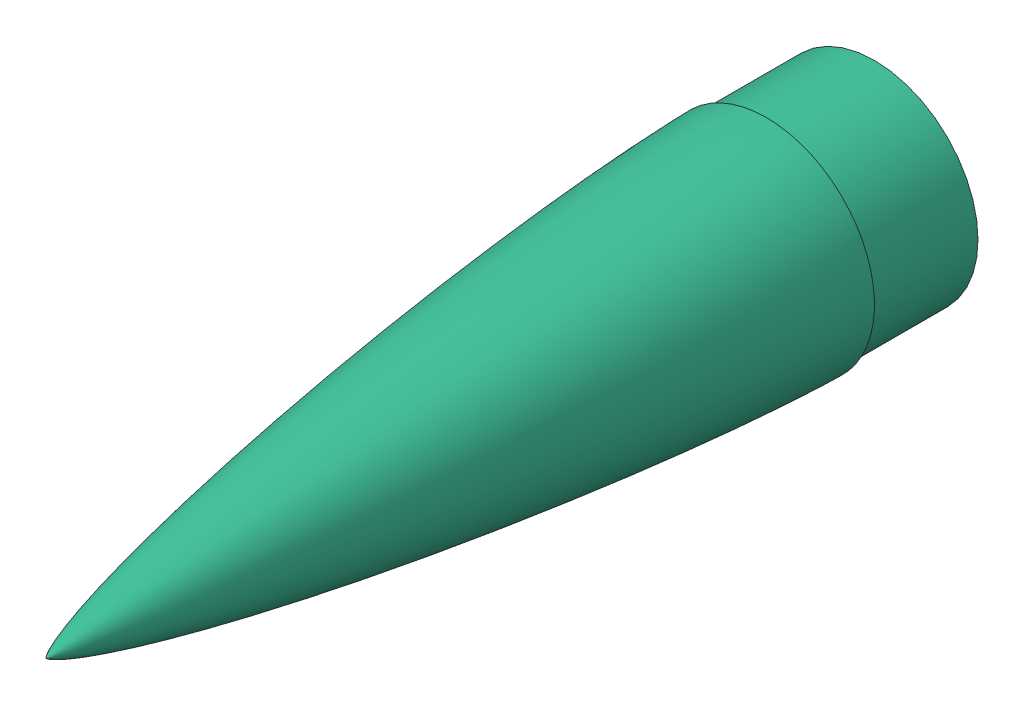
SolidWorks assembly Nosecone Assembly, configuration Default. Lengths in mm.
Overall size (152.4 152.4 590.12).
7 component instances, 7 part files, 13 mates.
Components (placement in the parent):
- 3112T31_Zinc-Plated Steel Round Eye Nut - for Lifting-1: 3112T31_Zinc-Plated Steel Round Eye Nut - for Lifting [3112T31] at (-62.4913 0 510.0607) x (0.999986 0.005369 0) z (-0.005369 0.999986 0) size (36.07 36.46 19.73)
- 90107A029_316 Stainless Steel Washer-1: 90107A029_316 Stainless Steel Washer [90107A029] at (-62.4913 0 546.986) size (15.88 15.88 1.27)
- 90322A658_High-Strength Steel Threaded Rod-1: 90322A658_High-Strength Steel Threaded Rod [90322A658] at (-62.4913 0 790.1916) x (-0.708492 -0.705719 0) z (0 0 1) size (7.33 6.42 560.63)
- 90630A110_High-Strength Steel Nylon-Insert Locknut-1: 90630A110_High-Strength Steel Nylon-Insert Locknut [90630A110] at (-62.4913 0 547.621) x (1 0 0) z (0 -1 0) size (11.11 8.31 12.83)
- 95462A029_Medium-Strength Steel Hex Nut-1: 95462A029_Medium-Strength Steel Hex Nut [95462A029] at (-62.4913 0 530.8728) x (0.99999 0.004487 0) z (0 0 1) size (11.11 12.75 6.32)
- LD-20-1: LD-20 [Default] at (-62.4913 0 1082.1485) x (0 0 -1) z (1 0 0) size (584.2 152.4 152.4)
- Nosecone Avionics Bulkhead-1: Nosecone Avionics Bulkhead [Default] at (-62.4913 0 546.351) x (1 0 0) z (0 1 0) size (139.7 12.7 139.7)
Mates (geometry in assembly coordinates):
- Concentric1: concentric anti-aligned: circle of 90322A658_High-Strength Steel Threaded Rod-1; circle of LD-20-1
- Coincident2: coincident aligned: plane of LD-20-1 through (-62.4913 0 1082.1485) normal (0 1 0)
- Tangent3: tangent: circle of 90322A658_High-Strength Steel Threaded Rod-1; face of LD-20-1
- Concentric2: concentric anti-aligned: cylinder of 90630A110_High-Strength Steel Nylon-Insert Locknut-1; cylinder of LD-20-1 through (-62.4913 0 574.1485) axis (0 0 -1) radius 69.85
- Coincident4: coincident anti-aligned: plane of 90107A029_316 Stainless Steel Washer-1 through (-62.4913 0 547.621) normal (0 0 1); plane of 90630A110_High-Strength Steel Nylon-Insert Locknut-1 through (-56.9351 3.2079 547.621) normal (0 0 -1)
- Concentric3: concentric aligned: circle of 90107A029_316 Stainless Steel Washer-1; circle of 90630A110_High-Strength Steel Nylon-Insert Locknut-1
- Concentric4: concentric aligned: circle of 3112T31_Zinc-Plated Steel Round Eye Nut - for Lifting-1; circle of 95462A029_Medium-Strength Steel Hex Nut-1
- Concentric5: concentric anti-aligned: cylinder of LD-20-1 through (-62.4913 0 574.1485) axis (0 0 -1) radius 69.85; cylinder of Nosecone Avionics Bulkhead-1 through (-62.4913 0 533.651) axis (0 0 1) radius 69.85
- Coincident6: coincident anti-aligned: plane of 90107A029_316 Stainless Steel Washer-1 through (-62.4913 0 546.351) normal (0 0 -1); plane of Nosecone Avionics Bulkhead-1 through (-62.4913 0 546.351) normal (0 0 1)
- Coincident7: coincident anti-aligned: plane of 95462A029_Medium-Strength Steel Hex Nut-1 through (-62.4913 0 533.651) normal (0 0 1); plane of Nosecone Avionics Bulkhead-1 through (-62.4913 0 533.651) normal (0 0 -1)
- Concentric6: concentric aligned: circle of 95462A029_Medium-Strength Steel Hex Nut-1; circle of Nosecone Avionics Bulkhead-1
- Coincident11: coincident anti-aligned: plane of 3112T31_Zinc-Plated Steel Round Eye Nut - for Lifting-1 through (-62.4913 0 528.0947) normal (0 0 1); plane of 95462A029_Medium-Strength Steel Hex Nut-1 through (-62.4913 0 528.0947) normal (0 0 -1)
- Coincident12: coincident aligned: plane of Nosecone Avionics Bulkhead-1 through (-62.4913 0 546.351) normal (0 1 0)
